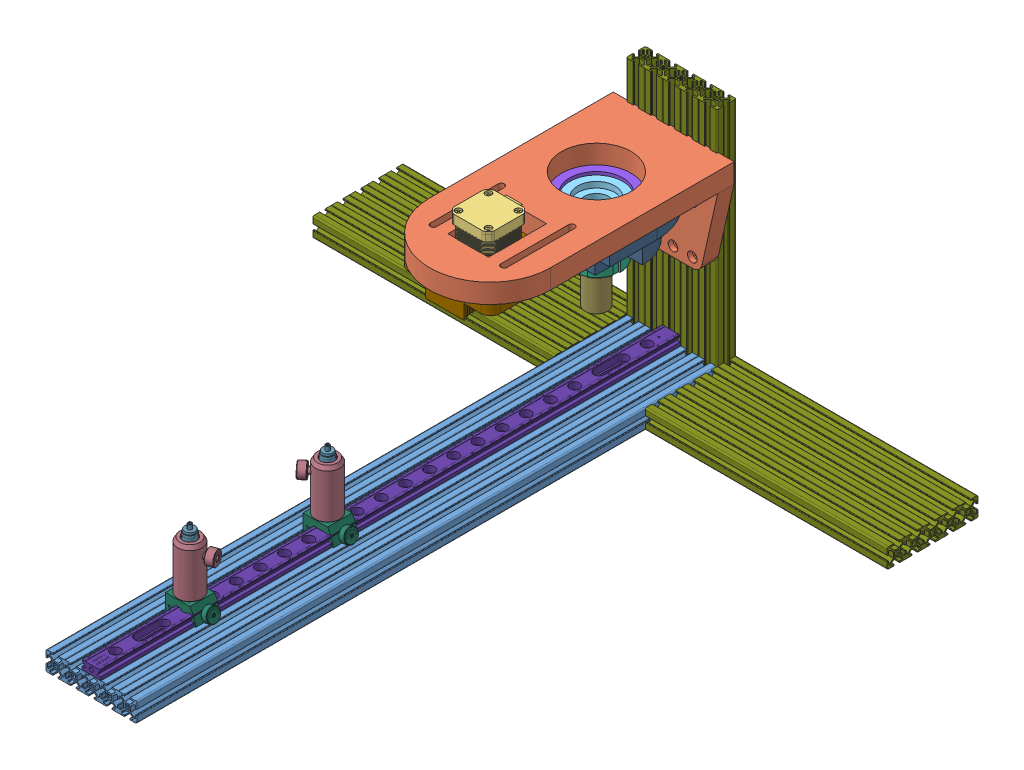
SolidWorks assembly OpenCALAssembly.v2, configuration Default. Lengths in mm.
Overall size (594 250 620.03).
24 component instances, 17 part files, 27 mates.
Components (placement in the parent):
- 20-2020-Black-25-CL.stp-1: 20-2020-Black-25-CL.stp [Default] at (5.4558 13.0651 39.4201) size (94 20 600)
- VerticalStageAssembly.v2-1: VerticalStageAssembly.v2 [Default] at (29.9175 152.6715 -478.4666) x (0 0 -1) z (1 0 0) size (252.5 140.51 125)
  - VerticalStage-1: VerticalStage [Default] at (83.6132 -98.677 -49.2178) size (252.5 100 125)
  - Nema17-1: Nema17 [Predeterminado] at (-108.1461 79.323 13.4322) x (0 0 1) z (1 0 0) size (42.3 64.5 47.8)
  - T5 Pulley-1: T5 Pulley [Predeterminado] at (-108.1461 32.623 13.4322) x (0 -1 0) z (0 0 1) size (14.8 16 16)
  - er32 x 34ths ToolHolderOpenCAL-1: er32 x 34ths ToolHolderOpenCAL [Default] at (-29.5654 28.1575 11.0488) x (0.967487 0 0.25292) z (0.25292 0 -0.967487) size (74 44.7 74)
  - ER32 COLLET NUT-1: ER32 COLLET NUT [Default] at (3.8533 8.9187 11.5736) x (0 -1 0) z (0.99027 0 0.13916) size (22.61 50 50)
  - ER32-20.step-1: ER32-20.step [Default] at (3.6132 -18.7965 13.2822) x (0.698361 0 0.715746) z (0 -1 0) size (32.96 32.96 40.01)
  - BallBearing-1: BallBearing [Default] at (3.6132 7.1575 13.2822) x (0.999353 0 0.035955) z (-0.035955 0 0.999353) size (72 9 72)
  - NemaAdjustableArm-2: NemaAdjustableArm [Default] at (-75.055 31.323 12.1091) size (90 25 95)
  - BallBearing-2: BallBearing [Default] at (3.6132 41.8575 13.2822) x (-0.59573 0 -0.803185) z (-0.803185 0 0.59573) size (72 9 72)
  - ColletStageHousing-1: ColletStageHousing [Default] at (3.6132 1.323 13.2822) x (0 1 0) z (0 0 -1) size (40 111.19 125)
  - Belt-1: Belt [Default] at (-108.6865 20.623 13.493) size (156.76 6 74)
  - Vial (20mm)-1: Vial (20mm) [Default] at (3.6132 -56.6823 13.2822) x (0.222456 0 0.974943) z (-0.974943 0 0.222456) size (23 41.5 23)
- PH50_M-Solidworks-1: PH50_M-Solidworks [Default] at (39.4918 57.7304 -72.239) x (-0.331511 0 -0.943451) z (0.943451 0 -0.331511) size (25 50.44 35.14)
- TR75_M-Solidworks-1: TR75_M-Solidworks [Default] at (34.6119 20.7616 -70.2602) x (0.667274 0 0.744812) z (-0.744812 0 0.667274) size (12.67 80.02 12.87)
- RC1-Solidworks-1: RC1-Solidworks [Default] at (53.5095 23.0651 -57.5602) x (0 0 -1) z (1 0 0) size (25.4 16.53 39.23)
- 20-2020-Black-25-CLShort.stp-1: 20-2020-Black-25-CLShort.stp [Default] at (-4.5442 13.0651 -496.5799) x (0 0 -1) z (1 0 0) size (94 20 250)
- 20-2020-Black-25-CLShort.stp-2: 20-2020-Black-25-CLShort.stp [Default] at (339.4558 13.0651 -496.5799) x (0 0 -1) z (1 0 0) size (94 20 250)
- PH50_M-Solidworks-2: PH50_M-Solidworks [Default] at (30.7203 57.7304 -209.1749) x (0.637938 0 0.770088) z (-0.770088 0 0.637938) size (25 50.44 35.14)
- TR75_M-Solidworks-2: TR75_M-Solidworks [Default] at (34.6119 19.9745 -212.7222) x (0.321219 0 0.947005) z (-0.947005 0 0.321219) size (12.67 80.02 12.87)
- RC1-Solidworks-2: RC1-Solidworks [Default] at (53.5095 23.0651 -200.0222) x (0 0 -1) z (1 0 0) size (25.4 16.53 39.23)
- RLA600_M-Solidworks-1: RLA600_M-Solidworks [Default] at (42.2404 28.1451 -260.5528) size (19.05 9.53 600)
- 20-2020-Black-25-CLShort.stp-4: 20-2020-Black-25-CLShort.stp [Default] at (79.4558 253.0651 -570.5799) x (-1 0 0) z (0 1 0) size (94 20 250)
Mates (geometry in assembly coordinates):
- Concentric1: concentric aligned: circle of PH50_M-Solidworks-1; cylinder of TR75_M-Solidworks-1 through (34.6119 95.7678 -70.2602) axis (0 1 0) radius 6.3373
- Concentric2: concentric anti-aligned: circle of PH50_M-Solidworks-1; circle of RC1-Solidworks-1
- Coincident4: coincident anti-aligned: plane of PH50_M-Solidworks-1 through (43.7754 38.5591 -44.1819) normal (0 -1 0); plane of RC1-Solidworks-1 through (21.9119 38.5591 -57.5602) normal (0 1 0)
- Parallel1: parallel aligned: plane of 20-2020-Black-25-CL.stp-1 through (-3.0442 4.5651 39.4201) normal (0 0 1); plane of RC1-Solidworks-1 through (21.9119 23.0651 -57.5602) normal (0 0 1)
- Coincident6: coincident aligned: line of 20-2020-Black-25-CL.stp-1 through (45.5938 23.0651 -560.5799) axis (0 0 1); line of RC1-Solidworks-1 through (45.5938 23.0651 -82.9602) axis (0 0 1)
- Coincident7: coincident anti-aligned: plane of 20-2020-Black-25-CL.stp-1 through (32.4558 23.0651 14.4201) normal (0 1 0); plane of RC1-Solidworks-1 through (21.9119 23.0651 -57.5602) normal (0 -1 0)
- Coincident13: coincident anti-aligned: plane of 20-2020-Black-25-CL.stp-1 through (89.4558 4.5651 14.4201) normal (1 0 0); plane of 20-2020-Black-25-CL.stp-3 through (89.4558 13.0651 -350.9237) normal (-1 0 0)
- Coincident15: coincident anti-aligned: plane of 20-2020-Black-25-CL.stp-1 through (-4.5442 21.5651 14.4201) normal (-1 0 0); plane of 20-2020-Black-25-CL.stp-4 through (-4.5442 4.5651 -488.0799) normal (1 0 0)
- Coincident19: coincident aligned: plane of 20-2020-Black-25-CLShort.stp-1 through (-29.5442 4.5651 -580.5799) normal (0 0 -1); plane of 20-2020-Black-25-CLShort.stp-2 through (314.4558 16.2031 -580.5799) normal (0 0 -1)
- Coincident20: coincident anti-aligned: plane of 20-2020-Black-25-CL.stp-1 through (89.4558 16.2031 14.4201) normal (1 0 0); plane of 20-2020-Black-25-CLShort.stp-2 through (89.4558 13.0651 -496.5799) normal (-1 0 0)
- Concentric3: concentric aligned: circle of PH50_M-Solidworks-2; cylinder of TR75_M-Solidworks-2 through (34.6119 94.9807 -212.7222) axis (0 1 0) radius 6.3373
- Concentric4: concentric anti-aligned: circle of PH50_M-Solidworks-2; circle of RC1-Solidworks-2
- Coincident21: coincident anti-aligned: plane of PH50_M-Solidworks-2 through (16.9784 38.5591 -234.0085) normal (0 -1 0); plane of RC1-Solidworks-2 through (21.9119 38.5591 -200.0222) normal (0 1 0)
- Parallel2: parallel aligned: plane of 20-2020-Black-25-CL.stp-1 through (-3.0442 4.5651 39.4201) normal (0 0 1); plane of RC1-Solidworks-2 through (21.9119 23.0651 -200.0222) normal (0 0 1)
- Coincident22: coincident aligned: line of 20-2020-Black-25-CL.stp-1 through (45.5938 23.0651 -560.5799) axis (0 0 1); line of RC1-Solidworks-2 through (45.5938 23.0651 -225.4222) axis (0 0 1)
- Coincident23: coincident anti-aligned: plane of 20-2020-Black-25-CL.stp-1 through (32.4558 23.0651 14.4201) normal (0 1 0); plane of RC1-Solidworks-2 through (21.9119 23.0651 -200.0222) normal (0 -1 0)
- Parallel4: parallel anti-aligned: line of 20-2020-Black-25-CL.stp-1 through (50.9558 23.0651 39.4201) axis (-1 0 0); line of RLA600_M-Solidworks-1 through (35.9158 23.3191 39.4472) axis (1 0 0)
- Coincident28: coincident anti-aligned: plane of 20-2020-Black-25-CL.stp-1 through (50.9558 23.0651 14.4201) normal (0 1 0); plane of RLA600_M-Solidworks-1 through (51.7654 23.0651 39.4472) normal (0 -1 0)
- Coincident36: coincident anti-aligned: plane of 20-2020-Black-25-CL.stp-1 through (5.4558 13.0651 -560.5799) normal (0 0 -1); plane of 20-2020-Black-25-CLShort.stp-4 through (-3.0442 228.0651 -560.5799) normal (0 0 1)
- Coincident37: coincident aligned: line of 20-2020-Black-25-CL.stp-1 through (-3.0442 3.0651 -560.5799) axis (1 0 0); line of 20-2020-Black-25-CLShort.stp-4 through (8.5938 3.0651 -560.5799) axis (1 0 0)
- Coincident38: coincident aligned: plane of 20-2020-Black-25-CL.stp-1 through (-4.5442 9.9271 14.4201) normal (-1 0 0); plane of 20-2020-Black-25-CLShort.stp-4 through (-4.5442 228.0651 -567.4419) normal (-1 0 0)
- Coincident45: coincident: point of VerticalStageAssembly.v2-1/VerticalStage-1; line of 20-2020-Black-25-CLShort.stp-4 through (89.4558 3.0651 -562.0799) axis (0 1 0)
- Parallel8: parallel aligned: plane of VerticalStageAssembly.v2-1/VerticalStage-1 through (105.6997 213.9945 -562.0799) normal (0 1 0); plane of 20-2020-Black-25-CLShort.stp-4 through (87.9558 253.0651 -579.0799) normal (0 1 0)
- Parallel9: parallel anti-aligned: plane of VerticalStageAssembly.v2-1/VerticalStage-1 through (105.6997 53.9945 -562.0799) normal (0 0 -1); plane of 20-2020-Black-25-CLShort.stp-4 through (-3.0442 228.0651 -560.5799) normal (0 0 1)
- Coincident48: coincident aligned: plane of 20-2020-Black-25-CLShort.stp-2 through (314.4558 16.2031 -580.5799) normal (0 0 -1); plane of 20-2020-Black-25-CLShort.stp-4 through (87.9558 228.0651 -580.5799) normal (0 0 -1)
- Coincident49: coincident aligned: plane of 20-2020-Black-25-CLShort.stp-2 through (314.4558 3.0651 -573.7179) normal (0 -1 0); plane of 20-2020-Black-25-CLShort.stp-4 through (79.4558 3.0651 -570.5799) normal (0 -1 0)
- Coincident50: coincident aligned: plane of 20-2020-Black-25-CLShort.stp-1 through (-29.5442 3.0651 -573.7179) normal (0 -1 0); plane of 20-2020-Black-25-CLShort.stp-4 through (79.4558 3.0651 -570.5799) normal (0 -1 0)
